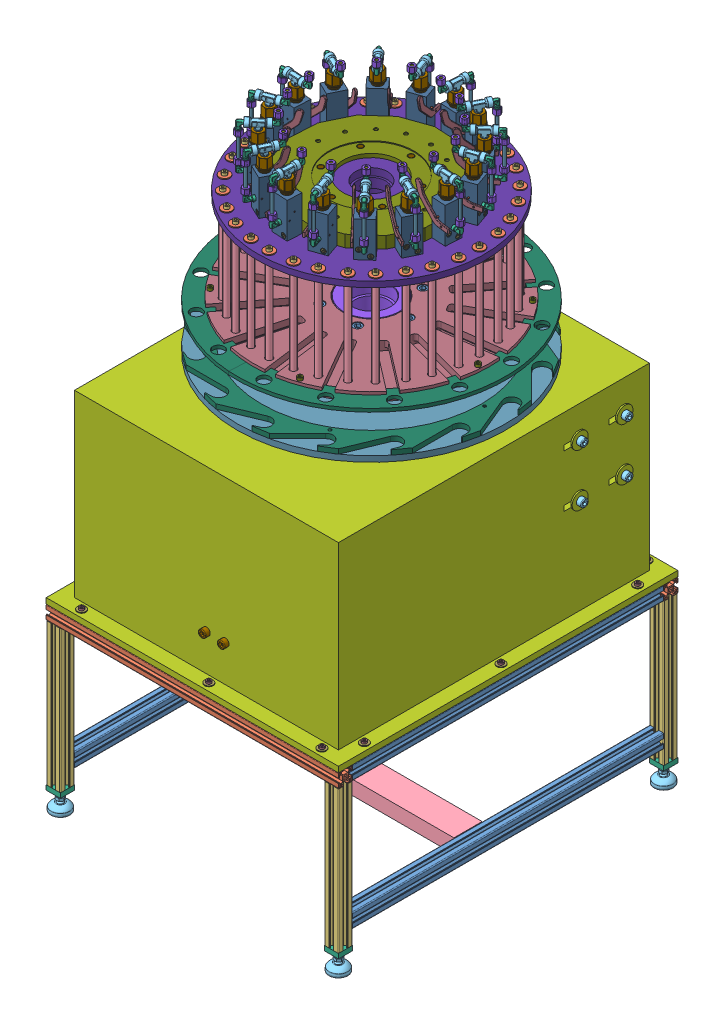
SolidWorks assembly Assieme_FINALE, configuration Default. Lengths in mm.
Overall size (778.63 1264.83 778.63).
659 component instances, 53 part files, 36 mates.
Components (placement in the parent):
- SupportoBase_Totale-2: SupportoBase_Totale [Default] at (4.0127 -14.4529 -3.9361) x (0 1 0) z (0 0 1) size (801.2 636.12 736.12)
  - Supporto_base_macchina-1: Supporto_base_macchina [Default] at origin size (378.2 636.12 736.12)
    - profilato_30x30_590-3: profilato_30x30_590 [Default] at (275.414 713.7262 -66.645) size (30 30 660)
    - profilato_30x30_590-5: profilato_30x30_590 [Default] at (275.414 123.7262 -66.645) size (30 30 660)
    - profilato_30x30_550-5: profilato_30x30_550 [Default] at (275.414 703.7262 -716.645) x (1 0 0) z (0 1 0) size (30 30 620)
    - profilato_30x30_550-6: profilato_30x30_550 [Default] at (275.414 703.7262 -26.645) x (1 0 0) z (0 1 0) size (30 30 620)
    - profilato_30x30_272-5: profilato_30x30_272 [Default] at (-16.586 123.7262 -716.645) x (0 0 1) z (-1 0 0) size (30 30 302)
    - profilato_30x30_272-6: profilato_30x30_272 [Default] at (-16.586 713.7262 -716.645) x (0 0 1) z (-1 0 0) size (30 30 302)
    - profilato_30x30_272-7: profilato_30x30_272 [Default] at (235.414 123.7262 -26.645) x (0 0 -1) z (1 0 0) size (30 30 302)
    - profilato_30x30_272-8: profilato_30x30_272 [Default] at (-16.586 713.7262 -26.645) x (0 0 1) z (-1 0 0) size (30 30 302)
    - profilo_U_60x30_490_supporto_base_macchina-1: profilo_U_60x30_490_supporto_base_macchina [Default] at (15.1 707.7262 -323.6583) x (0 0 1) z (0 -1 0) size (60 30 569)
    - profilato_30x30_590-6: profilato_30x30_590 [Default] at (3.414 123.7262 -66.645) size (30 30 660)
    - profilato_30x30_590-7: profilato_30x30_590 [Default] at (3.414 713.7262 -676.645) x (-1 0 0) z (0 0 -1) size (30 30 660)
    - 6322125-1: 6322125 [Default] at (-85.2818 713.7262 -26.645) x (0 0 -1) z (1 0 0) size (40 40 71.2)
    - 6322125-2: 6322125 [Default] at (-85.2818 713.7262 -716.645) x (0 0 -1) z (1 0 0) size (40 40 71.2)
    - 6322125-3: 6322125 [Default] at (-85.2818 123.7262 -26.645) x (0 -0.924225 -0.381849) z (1 0 0) size (40 40 71.2)
    - 6322125-4: 6322125 [Default] at (-85.2818 123.7262 -716.645) x (0 0 -1) z (1 0 0) size (40 40 71.2)
    - tappo_filettato_Supporto_base_macchina-1: tappo_filettato_Supporto_base_macchina [Default] at (-41.586 123.7262 -26.645) x (0 0 1) z (-1 0 0) size (30 30 10.37)
    - tappo_filettato_Supporto_base_macchina-2: tappo_filettato_Supporto_base_macchina [Default] at (-41.586 123.7262 -716.645) x (0 0 1) z (-1 0 0) size (30 30 10.37)
    - tappo_filettato_Supporto_base_macchina-3: tappo_filettato_Supporto_base_macchina [Default] at (-41.586 713.7262 -716.645) x (0 0 1) z (-1 0 0) size (30 30 10.37)
    - tappo_filettato_Supporto_base_macchina-4: tappo_filettato_Supporto_base_macchina [Default] at (-51.586 713.7262 -26.645) x (0 0 -1) z (1 0 0) size (30 30 10.37)
  - assieme_base-1: assieme_base [Default] at (466.8009 1138.7262 -472.0974) x (0 0 -1) z (0 -1 0) size (720 423 620)
    - Supporto di Base per macchina-1: Supporto di Base per macchina [Default] at (-460.4524 -176.3869 1030) size (720 403 620)
    - canotto di supporto-1: canotto di supporto [Default] at (-100.4524 134.8265 740) x (0 1 0) z (-0.866025 0 0.5) size (220 238 238)
    - m10 35mm-7: m10 35mm [ISO 4762 M10 x 35 - 35N] at (4.5476 246.6131 740) x (0 -1 0) z (1 0 0) size (45 16 16)
    - m10 35mm-8: m10 35mm [ISO 4762 M10 x 35 - 35N] at (-47.9524 246.6131 649.0673) x (0 -1 0) z (0.5 0 -0.866025) size (45 16 16)
    - m10 35mm-9: m10 35mm [ISO 4762 M10 x 35 - 35N] at (-152.9524 246.6131 649.0673) x (0 -1 0) z (-0.5 0 -0.866025) size (45 16 16)
    - m10 35mm-10: m10 35mm [ISO 4762 M10 x 35 - 35N] at (-205.4524 246.6131 740) x (0 -1 0) z (-1 0 0) size (45 16 16)
    - m10 35mm-11: m10 35mm [ISO 4762 M10 x 35 - 35N] at (-152.9524 246.6131 830.9327) x (0 -1 0) z (-0.5 0 0.866025) size (45 16 16)
    - m10 35mm-12: m10 35mm [ISO 4762 M10 x 35 - 35N] at (-47.9524 246.6131 830.9327) x (0 -1 0) z (0.5 0 0.866025) size (45 16 16)
    - Traversa di blocco albero-1: Traversa di blocco albero [Default] at (-100.4524 -86.3869 772.5) size (644 42 65)
    - m10 35mm-13: m10 35mm [ISO 4762 M10 x 35 - 35N] at (239.5476 -86.3869 760) x (-1 0 0) z (0 -1 0) size (45 16 16)
    - m10 35mm-16: m10 35mm [ISO 4762 M10 x 35 - 35N] at (239.5476 -86.3869 720) x (-1 0 0) z (0 -1 0) size (45 16 16)
    - m10 35mm-17: m10 35mm [ISO 4762 M10 x 35 - 35N] at (-440.4524 -86.3869 720) x (1 0 0) z (0 1 0) size (45 16 16)
    - m10 35mm-18: m10 35mm [ISO 4762 M10 x 35 - 35N] at (-440.4524 -86.3869 760) x (1 0 0) z (0 1 0) size (45 16 16)
  - DadoT-2: DadoT [Default] at (288.4104 668.7262 -716.645) x (0 0 -1) z (0 -1 0) size (16.5 6 8)
  - DadoT-9: DadoT [Default] at (288.4104 668.7262 -26.645) x (0 0 -1) z (0 -1 0) size (16.5 6 8)
  - DadoT-10: DadoT [Default] at (288.6104 713.7262 -661.645) x (0 1 0) z (0 0 -1) size (16.5 6 8)
  - DadoT-11: DadoT [Default] at (288.6104 713.7262 -371.645) x (0 1 0) z (0 0 -1) size (16.5 6 8)
  - DadoT-12: DadoT [Default] at (288.6104 713.7262 -81.645) x (0 1 0) z (0 0 -1) size (16.5 6 8)
  - DadoT-13: DadoT [Default] at (288.6104 123.7262 -661.645) x (0 1 0) z (0 0 -1) size (16.5 6 8)
  - DadoT-15: DadoT [Default] at (288.6104 123.7262 -371.645) x (0 1 0) z (0 0 -1) size (16.5 6 8)
  - DadoT-17: DadoT [Default] at (288.6104 123.7262 -81.645) x (0 1 0) z (0 0 -1) size (16.5 6 8)
  - RosettaM6-1: RosettaM6 [Washer ISO 7093 - 6] at (302.414 713.7262 -661.645) x (-1 0 0) z (0 0 1) size (1.6 18 18)
  - ViteM6-20-1: ViteM6-20 [ISO 4762 M6 x 20 - 20S] at (308.414 713.7262 -661.645) x (-1 0 0) z (0 0 1) size (26 10 10)
  - RosettaM6-2: RosettaM6 [Washer ISO 7093 - 6] at (302.414 668.7262 -716.645) x (-1 0 0) z (0 0 1) size (1.6 18 18)
  - ViteM6-20-2: ViteM6-20 [ISO 4762 M6 x 20 - 20S] at (308.414 668.7262 -716.645) x (-1 0 0) z (0 0 1) size (26 10 10)
  - RosettaM6-3: RosettaM6 [Washer ISO 7093 - 6] at (302.414 713.7262 -371.645) x (-1 0 0) z (0 0 1) size (1.6 18 18)
  - RosettaM6-4: RosettaM6 [Washer ISO 7093 - 6] at (302.414 713.7262 -81.645) x (-1 0 0) z (0 0 1) size (1.6 18 18)
  - ViteM6-20-3: ViteM6-20 [ISO 4762 M6 x 20 - 20S] at (308.414 713.7262 -371.645) x (-1 0 0) z (0 0 1) size (26 10 10)
  - ViteM6-20-4: ViteM6-20 [ISO 4762 M6 x 20 - 20S] at (308.414 713.7262 -81.645) x (-1 0 0) z (0 0 1) size (26 10 10)
  - RosettaM6-5: RosettaM6 [Washer ISO 7093 - 6] at (302.414 123.7262 -661.645) x (-1 0 0) z (0 0 1) size (1.6 18 18)
  - ViteM6-20-5: ViteM6-20 [ISO 4762 M6 x 20 - 20S] at (308.414 123.7262 -661.645) x (-1 0 0) z (0 0 1) size (26 10 10)
  - RosettaM6-6: RosettaM6 [Washer ISO 7093 - 6] at (302.414 123.7262 -371.645) x (-1 0 0) z (0 0 1) size (1.6 18 18)
  - RosettaM6-7: RosettaM6 [Washer ISO 7093 - 6] at (302.414 123.7262 -81.645) x (-1 0 0) z (0 0 1) size (1.6 18 18)
  - ViteM6-20-6: ViteM6-20 [ISO 4762 M6 x 20 - 20S] at (308.414 123.7262 -371.645) x (-1 0 0) z (0 0 1) size (26 10 10)
  - ViteM6-20-7: ViteM6-20 [ISO 4762 M6 x 20 - 20S] at (308.414 123.7262 -81.645) x (-1 0 0) z (0 0 1) size (26 10 10)
  - ViteM6-20-8: ViteM6-20 [ISO 4762 M6 x 20 - 20S] at (308.414 398.7262 -716.645) x (-1 0 0) z (0 0 1) size (26 10 10)
  - RosettaM6-8: RosettaM6 [Washer ISO 7093 - 6] at (302.414 398.7262 -716.645) x (-1 0 0) z (0 0 1) size (1.6 18 18)
  - DadoT-19: DadoT [Default] at (288.4104 398.7262 -716.645) x (0 0 -1) z (0 -1 0) size (16.5 6 8)
  - DadoT-20: DadoT [Default] at (288.4104 158.7262 -716.645) x (0 0 -1) z (0 -1 0) size (16.5 6 8)
  - RosettaM6-9: RosettaM6 [Washer ISO 7093 - 6] at (302.414 158.7262 -716.645) x (-1 0 0) z (0 0 1) size (1.6 18 18)
  - ViteM6-20-9: ViteM6-20 [ISO 4762 M6 x 20 - 20S] at (308.414 158.7262 -716.645) x (-1 0 0) z (0 0 1) size (26 10 10)
  - DadoT-21: DadoT [Default] at (288.4104 668.7262 -26.645) x (0 0 -1) z (0 -1 0) size (16.5 6 8)
  - RosettaM6-10: RosettaM6 [Washer ISO 7093 - 6] at (302.414 668.7262 -26.645) x (-1 0 0) z (0 0 1) size (1.6 18 18)
  - ViteM6-20-10: ViteM6-20 [ISO 4762 M6 x 20 - 20S] at (308.414 668.7262 -26.645) x (-1 0 0) z (0 0 1) size (26 10 10)
  - DadoT-22: DadoT [Default] at (288.4104 158.7262 -26.645) x (0 0 -1) z (0 -1 0) size (16.5 6 8)
  - RosettaM6-11: RosettaM6 [Washer ISO 7093 - 6] at (302.414 158.7262 -26.645) x (-1 0 0) z (0 0 1) size (1.6 18 18)
  - ViteM6-20-11: ViteM6-20 [ISO 4762 M6 x 20 - 20S] at (308.414 158.7262 -26.645) x (-1 0 0) z (0 0 1) size (26 10 10)
  - ViteM6-20-12: ViteM6-20 [ISO 4762 M6 x 20 - 20S] at (308.414 398.7262 -26.645) x (-1 0 0) z (0 0 1) size (26 10 10)
  - RosettaM6-12: RosettaM6 [Washer ISO 7093 - 6] at (302.414 398.7262 -26.645) x (-1 0 0) z (0 0 1) size (1.6 18 18)
  - DadoT-23: DadoT [Default] at (288.4104 398.7262 -26.645) x (0 0 -1) z (0 -1 0) size (16.5 6 8)
- motoriduttore-1: motoriduttore [Default] at (-164.7135 275.9611 -1179.5811) x (0 0 1) z (-1 0 0) size (200 160 175)
- Assieme_Riduttore-1: Assieme_Riduttore [Default] at (-346.4148 520.923 -401.8673) x (0 1 0) z (0.342115 0 -0.939658) size (226 168.82 169.04)
  - AlberoRiduttore-1: AlberoRiduttore [Default] at (-61.6906 7.4655 211) size (201 29 29)
  - linguetta_uni6604_b_8x7x50-1: linguetta_uni6604_b_8x7x50 [Default] at (-116.7419 7.4655 226) x (1 0 0) z (0 1 0) size (50 7 8)
  - linguetta_uni6604_b_8x7x35-1: linguetta_uni6604_b_8x7x35 [Default] at (-33.7419 7.4655 226.5) x (1 0 0) z (0 1 0) size (35 7 8)
  - linguetta_uni6604_b_8x7x35-2: linguetta_uni6604_b_8x7x35 [Default] at (41.2581 7.4655 226.5) x (1 0 0) z (0 1 0) size (35 7 8)
  - ASSIEME-LASS-90-VERS-B-O-25-3D.step-1: ASSIEME-LASS-90-VERS-B-O-25-3D.step [Default] at (-111.3519 -70.5563 279.3493) x (-1 0 0) z (0 0.707107 -0.707107) size (64.28 105 105)
  - Rondella di fermo-1: Rondella di fermo [Default] at (-122.7419 7.4655 211) x (0 0.707107 -0.707107) z (-1 0 0) size (36 36 3)
  - M8 25 mm-1: M8 25 mm [ISO 4762 M8 x 25 - 25N] at (92.2581 7.4655 211) x (-1 0 0) z (0 1 0) size (33 13 13)
  - M8 25 mm-2: M8 25 mm [ISO 4762 M8 x 25 - 25N] at (-133.7419 7.4655 211) x (1 0 0) z (0 -0.707107 0.707107) size (33 13 13)
  - M6 16mm-3: M6 16mm [ISO 4762 M6 x 16 - 16N] at (-44.8119 40.5589 196.8286) x (-1 0 0) z (0 0.935687 0.352831) size (22 10 10)
  - M6 16mm-14: M6 16mm [ISO 4762 M6 x 16 - 16N] at (-44.8119 11.7394 175.2546) x (-1 0 0) z (0 0.773404 -0.633913) size (22 10 10)
  - M6 16mm-15: M6 16mm [ISO 4762 M6 x 16 - 16N] at (-44.8119 -21.354 189.426) x (-1 0 0) z (0 -0.162283 -0.986744) size (22 10 10)
  - M6 16mm-16: M6 16mm [ISO 4762 M6 x 16 - 16N] at (-44.8119 -25.6279 225.1714) x (-1 0 0) z (0 -0.935687 -0.352831) size (22 10 10)
  - M6 16mm-17: M6 16mm [ISO 4762 M6 x 16 - 16N] at (-44.8119 3.1916 246.7454) x (-1 0 0) z (0 -0.773404 0.633913) size (22 10 10)
  - M6 16mm-18: M6 16mm [ISO 4762 M6 x 16 - 16N] at (-44.8119 36.285 232.574) x (-1 0 0) z (0 0.162283 0.986744) size (22 10 10)
  - Parte1^Assieme_Riduttore-1: Parte1^Assieme_Riduttore [Default] at origin (virtual)
  - ruota dentata m22-4: ruota dentata m22 [Chain wheel ISO - 22Z 10A-1 --22SA36.0N] at (-59.7419 7.4655 211) x (1 0 0) z (0 -0.599278 0.800541) size (8.93 120.13 121.23)
  - Rondella di fermo-2: Rondella di fermo [Default] at (84.2581 7.4655 211) x (0 0 1) z (-1 0 0) size (36 36 3)
- socket head cap screw_iso-1: socket head cap screw_iso [ISO 4762 M10 x 40 - 40N] at (-121.7135 603.4611 -555.5811) x (-1 0 0) z (0 -0.924225 -0.381849) size (50 16 16)
- socket head cap screw_iso-2: socket head cap screw_iso [ISO 4762 M10 x 40 - 40N] at (-121.7135 492.4611 -555.5811) x (-1 0 0) z (0 0 1) size (50 16 16)
- socket head cap screw_iso-3: socket head cap screw_iso [ISO 4762 M10 x 40 - 40N] at (-121.7135 603.4611 -650.5811) x (-1 0 0) z (0 0 1) size (50 16 16)
- socket head cap screw_iso-4: socket head cap screw_iso [ISO 4762 M10 x 40 - 40N] at (-121.7135 492.4611 -650.5811) x (-1 0 0) z (0 0 1) size (50 16 16)
- hex nut style 2 gradeab_iso-1: hex nut style 2 gradeab_iso [ISO - 4033 - M10 - W - N] at (-174.0135 603.4611 -650.5811) x (0 0 1) z (-1 0 0) size (16 18.48 9.3)
- hex nut style 2 gradeab_iso-2: hex nut style 2 gradeab_iso [ISO - 4033 - M10 - W - N] at (-174.0135 603.4611 -555.5811) x (0 0 1) z (-1 0 0) size (16 18.48 9.3)
- hex nut style 2 gradeab_iso-3: hex nut style 2 gradeab_iso [ISO - 4033 - M10 - W - N] at (-174.0135 492.4611 -650.5811) x (0 0 1) z (-1 0 0) size (16 18.48 9.3)
- hex nut style 2 gradeab_iso-4: hex nut style 2 gradeab_iso [ISO - 4033 - M10 - W - N] at (-174.0135 492.4611 -555.5811) x (0 0 1) z (-1 0 0) size (16 18.48 9.3)
- plain washer xlarge grade c_iso-1: plain washer xlarge grade c_iso [Washer ISO 7094 - 10] at (-134.7135 603.4611 -555.5811) x (-1 0 0) z (0 0.924225 0.381849) size (3 34 34)
- plain washer xlarge grade c_iso-2: plain washer xlarge grade c_iso [Washer ISO 7094 - 10] at (-134.7135 492.4611 -555.5811) x (-1 0 0) z (0 0 1) size (3 34 34)
- plain washer xlarge grade c_iso-3: plain washer xlarge grade c_iso [Washer ISO 7094 - 10] at (-134.7135 492.4611 -650.5811) x (-1 0 0) z (0 0 1) size (3 34 34)
- plain washer xlarge grade c_iso-4: plain washer xlarge grade c_iso [Washer ISO 7094 - 10] at (-134.7135 603.4611 -650.5811) x (-1 0 0) z (0 0 1) size (3 34 34)
- assieme parte rotante-1: assieme parte rotante [Default] at (-376.3498 623.9178 -790.5811) x (0 1 0) z (0 0 1) size (749.63 778.63 778.63)
  - albero rotazione piatti-1: albero rotazione piatti [Default] at (60.413 18.3637 415) size (415 200 200)
  - seger 100mm-1: seger 100mm [KS 1336 E - 100] at (-146.4567 18.3637 415) x (0 0 -1) z (1 0 0) size (107.55 112.98 3)
  - SKF - 6020 - 20,DE,NC,20_68-1: SKF - 6020 - 20,DE,NC,20_68 [SKF - 6020 - 20,DE,NC,20_68] at (-131.4567 18.3637 415) x (1 0 0) z (0 -0.434476 -0.900684) size (24 150 150)
  - calettatore d95-1: calettatore d95 [Default] at (-173.8867 18.3637 415) size (39.5 135 135)
  - Chain wheel ISO - 50Z 10A-1-1: Chain wheel ISO - 50Z 10A-1 [Chain wheel ISO - 50Z 10A-1 --50SB120H25L95.0N] at (-164.8867 18.3637 415) size (28.93 262.06 262.51)
  - Disco supporto montaggio e Colonne-1: Disco supporto montaggio e Colonne [Default] at (204.0433 18.3637 415) x (0 -0.866025 -0.5) z (1 0 0) size (499.6 499.6 29)
  - SKF - 6020 - 20,DE,NC,20_68-2: SKF - 6020 - 20,DE,NC,20_68 [SKF - 6020 - 20,DE,NC,20_68] at (62.0433 18.3637 415) x (1 0 0) z (0 -0.432628 -0.901573) size (24 150 150)
  - piatto rotante porta tappi-1: piatto rotante porta tappi [Default] at (99.0433 18.3637 415) x (0 0 -1) z (1 0 0) size (570 570 20.57)
  - disco trasportatore tappi 31-1: disco trasportatore tappi 31 [Default] at (111.0433 18.3637 415) x (0 0.5 -0.866025) z (1 0 0) size (570 570 10.42)
  - Distributore Rotante-1: Distributore Rotante [Default] at (425.0433 18.3637 415) x (0 -0.055301 -0.99847) z (1 0 0) size (310 310 25.54)
  - disco trascinato porta distributore vuoto-1: disco trascinato porta distributore vuoto [Default] at (400.0433 18.3637 415) x (0 0.055301 0.99847) z (-1 0 0) size (480 480 50)
  - m12 35mm-1: m12 35mm [ISO 4762 M12 x 35 - 35N] at (376.0433 -53.0243 378.8925) x (1 0 0) z (0 -0.5 0.866025) size (47 18 18)
  - m12 90mm-3: m12 90mm [ISO 4762 M12 x 90 - 90N] at (203.0433 -21.6363 345.718) x (-1 0 0) z (0 -0.5 0.866025) size (102 18 18)
  - rondella m6 22mm-1: rondella m6 22mm [Washer ISO 7094 - 6] at (99.0433 -101.6363 207.1539) x (1 0 0) z (0 -1 0) size (2 22 22)
  - M6 20mm-1: M6 20mm [ISO 4762 M6 x 20 - 20N] at (91.0433 -101.6363 207.1539) x (1 0 0) z (0 0.5 0.866025) size (26 10 10)
  - m12 35mm-2: m12 35mm [ISO 4762 M12 x 35 - 35N] at (376.0433 13.9397 335.1224) x (1 0 0) z (0 -1 0) size (47 18 18)
  - m12 35mm-3: m12 35mm [ISO 4762 M12 x 35 - 35N] at (376.0433 85.3277 371.2299) x (1 0 0) z (0 -0.5 -0.866025) size (47 18 18)
  - m12 35mm-4: m12 35mm [ISO 4762 M12 x 35 - 35N] at (376.0433 89.7517 451.1075) x (1 0 0) z (0 0.5 -0.866025) size (47 18 18)
  - m12 35mm-5: m12 35mm [ISO 4762 M12 x 35 - 35N] at (376.0433 22.7877 494.8776) x (1 0 0) z (0 1 0) size (47 18 18)
  - m12 35mm-6: m12 35mm [ISO 4762 M12 x 35 - 35N] at (376.0433 -48.6003 458.7701) x (1 0 0) z (0 0.5 0.866025) size (47 18 18)
  - rondella m6 22mm-2: rondella m6 22mm [Washer ISO 7094 - 6] at (99.0433 138.3637 207.1539) x (1 0 0) z (0 -0.5 -0.866025) size (2 22 22)
  - rondella m6 22mm-3: rondella m6 22mm [Washer ISO 7094 - 6] at (99.0433 258.3637 415) x (1 0 0) z (0 0.5 -0.866025) size (2 22 22)
  - rondella m6 22mm-4: rondella m6 22mm [Washer ISO 7094 - 6] at (99.0433 138.3637 622.8461) x (1 0 0) z (0 1 0) size (2 22 22)
  - rondella m6 22mm-5: rondella m6 22mm [Washer ISO 7094 - 6] at (99.0433 -101.6363 622.8461) x (1 0 0) z (0 0.5 0.866025) size (2 22 22)
  - rondella m6 22mm-6: rondella m6 22mm [Washer ISO 7094 - 6] at (99.0433 -221.6363 415) x (1 0 0) z (0 -0.5 0.866025) size (2 22 22)
  - M6 20mm-2: M6 20mm [ISO 4762 M6 x 20 - 20N] at (91.0433 138.3637 207.1539) x (1 0 0) z (0 -0.5 0.866025) size (26 10 10)
  - M6 20mm-3: M6 20mm [ISO 4762 M6 x 20 - 20N] at (91.0433 258.3637 415) x (1 0 0) z (0 -1 0) size (26 10 10)
  - M6 20mm-4: M6 20mm [ISO 4762 M6 x 20 - 20N] at (91.0433 138.3637 622.8461) x (1 0 0) z (0 -0.5 -0.866025) size (26 10 10)
  - M6 20mm-5: M6 20mm [ISO 4762 M6 x 20 - 20N] at (91.0433 -101.6363 622.8461) x (1 0 0) z (0 0.5 -0.866025) size (26 10 10)
  - M6 20mm-6: M6 20mm [ISO 4762 M6 x 20 - 20N] at (91.0433 -221.6363 415) x (1 0 0) z (0 1 0) size (26 10 10)
  - m12 90mm-4: m12 90mm [ISO 4762 M12 x 90 - 90N] at (203.0433 58.3637 345.718) x (-1 0 0) z (0 -1 0) size (102 18 18)
  - m12 90mm-5: m12 90mm [ISO 4762 M12 x 90 - 90N] at (203.0433 98.3637 415) x (-1 0 0) z (0 -0.5 -0.866025) size (102 18 18)
  - m12 90mm-6: m12 90mm [ISO 4762 M12 x 90 - 90N] at (203.0433 58.3637 484.282) x (-1 0 0) z (0 0.5 -0.866025) size (102 18 18)
  - m12 90mm-7: m12 90mm [ISO 4762 M12 x 90 - 90N] at (203.0433 -21.6363 484.282) x (-1 0 0) z (0 1 0) size (102 18 18)
  - m12 90mm-8: m12 90mm [ISO 4762 M12 x 90 - 90N] at (203.0433 -61.6363 415) x (-1 0 0) z (0 0.5 0.866025) size (102 18 18)
  - asta scorrimento carello-1: asta scorrimento carello [Default] at (287.5433 70.1437 197.9013) x (0 0 -1) z (1 0 0) size (12 12 225)
  - rondella m6 22mm-7: rondella m6 22mm [Washer ISO 7094 - 6] at (175.0433 70.1437 197.9013) x (1 0 0) z (0 -1 0) size (2 22 22)
  - M6 16mm-1: M6 16mm [ISO 4762 M6 x 16 - 16N] at (167.0433 70.1437 197.9013) size (22 10 10)
  - M6 16mm-2: M6 16mm [ISO 4762 M6 x 16 - 16N] at (408.0433 70.1437 197.9013) x (-1 0 0) z (0 0 -1) size (22 10 10)
  - rondella m6 22mm-8: rondella m6 22mm [Washer ISO 7094 - 6] at (400.0433 70.1437 197.9013) x (-1 0 0) z (0 1 0) size (2 22 22)
  - rondella m6 22mm-9: rondella m6 22mm [Washer ISO 7094 - 6] at (175.0433 24.5373 191.8971) x (1 0 0) z (0 -0.965926 -0.258819) size (2 22 22)
  - M6 16mm-3: M6 16mm [ISO 4762 M6 x 16 - 16N] at (167.0433 24.5373 191.8971) x (1 0 0) z (0 0.258819 -0.965926) size (22 10 10)
  - asta scorrimento carello-2: asta scorrimento carello [Default] at (287.5433 24.5373 191.8971) x (0 0.258819 -0.965926) z (-1 0 0) size (12 12 225)
  - rondella m6 22mm-10: rondella m6 22mm [Washer ISO 7094 - 6] at (400.0433 24.5373 191.8971) x (-1 0 0) z (0 0.965926 0.258819) size (2 22 22)
  - M6 16mm-4: M6 16mm [ISO 4762 M6 x 16 - 16N] at (408.0433 24.5373 191.8971) x (-1 0 0) z (0 -0.258819 0.965926) size (22 10 10)
  - AssiemeValvola-1: AssiemeValvola [Default] at (515.3257 74.6348 254.5832) x (0 -0.331007 0.943628) z (0 0.943628 0.331007) size (90.26 138.63 38)
    - RaccordoT-1: RaccordoT [Default] at origin size (43 29.75 16.5)
    - Raccordo a L-1: Raccordo a L [Default] at (-30 0 0) x (0 -1 0) z (0 0 -1) size (28.34 25.51 14.01)
      - 1809_06_10_01-1: 1809_06_10_01 [Default] at origin size (22.49 23 10)
      - 1809_06_10_02-1: 1809_06_10_02 [Default] at origin size (6.5 8.5 8.5)
      - 1809_06_10_03-1: 1809_06_10_03 [Default] at origin size (11.02 15.01 14.01)
    - Raccordo a L-2: Raccordo a L [Default] at (30 0 0) x (0 1 0) z (0 0 -1) size (28.34 25.51 14.01)
      - 1809_06_10_01-1: 1809_06_10_01 [Default] at origin size (22.49 23 10)
      - 1809_06_10_02-1: 1809_06_10_02 [Default] at origin size (6.5 8.5 8.5)
      - 1809_06_10_03-1: 1809_06_10_03 [Default] at origin size (11.02 15.01 14.01)
    - TappoChiusura-1: TappoChiusura [Default] at (0 -32 0) x (0 -1 0) z (0 0 1) size (38.28 26.74 26.74)
    - CorpoValvola-1: CorpoValvola [Default] at (-15 -115.2824 0) size (30 75 34)
    - Raccordo a L-3: Raccordo a L [Default] at (-30 -88.2824 0) x (0 1 0) z (0 0 1) size (28.34 25.51 14.01)
      - 1809_06_10_01-1: 1809_06_10_01 [Default] at origin size (22.49 23 10)
      - 1809_06_10_02-1: 1809_06_10_02 [Default] at origin size (6.5 8.5 8.5)
      - 1809_06_10_03-1: 1809_06_10_03 [Default] at origin size (11.02 15.01 14.01)
    - Spina_3x38-1: Spina_3x38 [Default] at (0 -68.2824 -21) x (-1 0 0) z (0 0 1) size (3 3 38)
    - Spina_3x38-2: Spina_3x38 [Default] at (-10 -80.2824 -21) x (0.996193 0.087174 0) z (0 0 1) size (3 3 38)
    - M5 40mm-3: M5 40mm [ISO 4762 M5 x 40 - 40N] at (-14.6 -108.7824 9) size (45 8.5 8.5)
    - M5 40mm-2: M5 40mm [ISO 4762 M5 x 40 - 40N] at (-14.6 -96.7824 -9) size (45 8.5 8.5)
    - LevaValvola-1: LevaValvola [Default] at (-24.507 -86.571 -17) x (0.996193 0.087174 0) z (0 0 1) size (77.55 60.2 4)
    - Tubo-1: Tubo [Default] at (-30 -15.9665 0) x (1 0 0) z (0 -1 0) size (6 6 56.4)
  - M6 16mm-5: M6 16mm [ISO 4762 M6 x 16 - 16N] at (167.0433 -16.8778 194.6116) x (1 0 0) z (0 0.382683 0.92388) size (22 10 10)
  - M6 16mm-6: M6 16mm [ISO 4762 M6 x 16 - 16N] at (167.0433 -98.5342 224.874) x (1 0 0) z (0 0.707107 0.707107) size (22 10 10)
  - M6 16mm-7: M6 16mm [ISO 4762 M6 x 16 - 16N] at (167.0433 -162.3939 284.0814) x (1 0 0) z (0 0.92388 0.382683) size (22 10 10)
  - M6 16mm-8: M6 16mm [ISO 4762 M6 x 16 - 16N] at (167.0433 -198.735 363.22) x (1 0 0) z (0 1 0) size (22 10 10)
  - M6 16mm-9: M6 16mm [ISO 4762 M6 x 16 - 16N] at (167.0433 -202.0247 450.2415) x (1 0 0) z (0 0.92388 -0.382683) size (22 10 10)
  - M6 16mm-10: M6 16mm [ISO 4762 M6 x 16 - 16N] at (167.0433 -171.7623 531.8979) x (1 0 0) z (0 0.707107 -0.707107) size (22 10 10)
  - M6 16mm-11: M6 16mm [ISO 4762 M6 x 16 - 16N] at (167.0433 -112.5549 595.7576) x (1 0 0) z (0 0.382683 -0.92388) size (22 10 10)
  - M6 16mm-12: M6 16mm [ISO 4762 M6 x 16 - 16N] at (167.0433 -33.4163 632.0987) x (1 0 0) z (0 0 -1) size (22 10 10)
  - M6 16mm-13: M6 16mm [ISO 4762 M6 x 16 - 16N] at (167.0433 53.6052 635.3884) x (1 0 0) z (0 -0.382683 -0.92388) size (22 10 10)
  - M6 16mm-14: M6 16mm [ISO 4762 M6 x 16 - 16N] at (167.0433 135.2616 605.126) x (1 0 0) z (0 -0.707107 -0.707107) size (22 10 10)
  - M6 16mm-15: M6 16mm [ISO 4762 M6 x 16 - 16N] at (167.0433 199.1213 545.9186) x (1 0 0) z (0 -0.92388 -0.382683) size (22 10 10)
  - M6 16mm-16: M6 16mm [ISO 4762 M6 x 16 - 16N] at (167.0433 235.4624 466.78) x (1 0 0) z (0 -1 0) size (22 10 10)
  - M6 16mm-17: M6 16mm [ISO 4762 M6 x 16 - 16N] at (167.0433 238.7521 379.7585) x (1 0 0) z (0 -0.92388 0.382683) size (22 10 10)
  - M6 16mm-18: M6 16mm [ISO 4762 M6 x 16 - 16N] at (167.0433 208.4897 298.1021) x (1 0 0) z (0 -0.707107 0.707107) size (22 10 10)
  - M6 16mm-19: M6 16mm [ISO 4762 M6 x 16 - 16N] at (167.0433 149.2823 234.2424) x (1 0 0) z (0 -0.382683 0.92388) size (22 10 10)
  - rondella m6 22mm-11: rondella m6 22mm [Washer ISO 7094 - 6] at (175.0433 -16.8778 194.6116) x (1 0 0) z (0 -0.92388 0.382683) size (2 22 22)
  - rondella m6 22mm-12: rondella m6 22mm [Washer ISO 7094 - 6] at (175.0433 -98.5342 224.874) x (1 0 0) z (0 -0.707107 0.707107) size (2 22 22)
  - rondella m6 22mm-13: rondella m6 22mm [Washer ISO 7094 - 6] at (175.0433 -162.3939 284.0814) x (1 0 0) z (0 -0.382683 0.92388) size (2 22 22)
  - rondella m6 22mm-14: rondella m6 22mm [Washer ISO 7094 - 6] at (175.0433 -198.735 363.22) size (2 22 22)
  - rondella m6 22mm-15: rondella m6 22mm [Washer ISO 7094 - 6] at (175.0433 -202.0247 450.2415) x (1 0 0) z (0 0.382683 0.92388) size (2 22 22)
  - rondella m6 22mm-16: rondella m6 22mm [Washer ISO 7094 - 6] at (175.0433 -171.7623 531.8979) x (1 0 0) z (0 0.707107 0.707107) size (2 22 22)
  - rondella m6 22mm-17: rondella m6 22mm [Washer ISO 7094 - 6] at (175.0433 -112.5549 595.7576) x (1 0 0) z (0 0.92388 0.382683) size (2 22 22)
  - rondella m6 22mm-18: rondella m6 22mm [Washer ISO 7094 - 6] at (175.0433 -33.4163 632.0987) x (1 0 0) z (0 1 0) size (2 22 22)
  - rondella m6 22mm-19: rondella m6 22mm [Washer ISO 7094 - 6] at (175.0433 53.6052 635.3884) x (1 0 0) z (0 0.92388 -0.382683) size (2 22 22)
  - rondella m6 22mm-20: rondella m6 22mm [Washer ISO 7094 - 6] at (175.0433 135.2616 605.126) x (1 0 0) z (0 0.707107 -0.707107) size (2 22 22)
  - rondella m6 22mm-21: rondella m6 22mm [Washer ISO 7094 - 6] at (175.0433 199.1213 545.9186) x (1 0 0) z (0 0.382683 -0.92388) size (2 22 22)
  - rondella m6 22mm-22: rondella m6 22mm [Washer ISO 7094 - 6] at (175.0433 235.4624 466.78) x (1 0 0) z (0 0 -1) size (2 22 22)
  - rondella m6 22mm-23: rondella m6 22mm [Washer ISO 7094 - 6] at (175.0433 238.7521 379.7585) x (1 0 0) z (0 -0.382683 -0.92388) size (2 22 22)
  - rondella m6 22mm-24: rondella m6 22mm [Washer ISO 7094 - 6] at (175.0433 208.4897 298.1021) x (1 0 0) z (0 -0.707107 -0.707107) size (2 22 22)
  - rondella m6 22mm-25: rondella m6 22mm [Washer ISO 7094 - 6] at (175.0433 149.2823 234.2424) x (1 0 0) z (0 -0.92388 -0.382683) size (2 22 22)
  - asta scorrimento carello-3: asta scorrimento carello [Default] at (287.5433 -16.8778 194.6116) x (0 -0.382683 -0.92388) z (1 0 0) size (12 12 225)
  - asta scorrimento carello-4: asta scorrimento carello [Default] at (287.5433 -98.5342 224.874) x (0 -0.707107 -0.707107) z (1 0 0) size (12 12 225)
  - asta scorrimento carello-5: asta scorrimento carello [Default] at (287.5433 -162.3939 284.0814) x (0 -0.92388 -0.382683) z (1 0 0) size (12 12 225)
  - asta scorrimento carello-6: asta scorrimento carello [Default] at (287.5433 -198.735 363.22) x (0 -1 0) z (1 0 0) size (12 12 225)
  - asta scorrimento carello-7: asta scorrimento carello [Default] at (287.5433 -202.0247 450.2415) x (0 -0.92388 0.382683) z (1 0 0) size (12 12 225)
  - asta scorrimento carello-8: asta scorrimento carello [Default] at (287.5433 -171.7623 531.8979) x (0 -0.707107 0.707107) z (1 0 0) size (12 12 225)
  - asta scorrimento carello-9: asta scorrimento carello [Default] at (287.5433 -112.5549 595.7576) x (0 -0.382683 0.92388) z (1 0 0) size (12 12 225)
  - asta scorrimento carello-10: asta scorrimento carello [Default] at (287.5433 -33.4163 632.0987) x (0 0 1) z (1 0 0) size (12 12 225)
  - asta scorrimento carello-11: asta scorrimento carello [Default] at (287.5433 53.6052 635.3884) x (0 0.382683 0.92388) z (1 0 0) size (12 12 225)
  - asta scorrimento carello-12: asta scorrimento carello [Default] at (287.5433 135.2616 605.126) x (0 0.707107 0.707107) z (1 0 0) size (12 12 225)
  - asta scorrimento carello-13: asta scorrimento carello [Default] at (287.5433 199.1213 545.9186) x (0 0.92388 0.382683) z (1 0 0) size (12 12 225)
  - asta scorrimento carello-14: asta scorrimento carello [Default] at (287.5433 235.4624 466.78) x (0 1 0) z (1 0 0) size (12 12 225)
  - asta scorrimento carello-15: asta scorrimento carello [Default] at (287.5433 238.7521 379.7585) x (0 0.92388 -0.382683) z (1 0 0) size (12 12 225)
  - asta scorrimento carello-16: asta scorrimento carello [Default] at (287.5433 208.4897 298.1021) x (0 0.707107 -0.707107) z (1 0 0) size (12 12 225)
  - asta scorrimento carello-17: asta scorrimento carello [Default] at (287.5433 149.2823 234.2424) x (0 0.382683 -0.92388) z (1 0 0) size (12 12 225)
  - M6 16mm-20: M6 16mm [ISO 4762 M6 x 16 - 16N] at (408.0433 -16.8778 194.6116) x (-1 0 0) z (0 -0.382683 -0.92388) size (22 10 10)
  - M6 16mm-21: M6 16mm [ISO 4762 M6 x 16 - 16N] at (408.0433 -98.5342 224.874) x (-1 0 0) z (0 -0.707107 -0.707107) size (22 10 10)
  - M6 16mm-22: M6 16mm [ISO 4762 M6 x 16 - 16N] at (408.0433 -162.3939 284.0814) x (-1 0 0) z (0 -0.92388 -0.382683) size (22 10 10)
  - M6 16mm-23: M6 16mm [ISO 4762 M6 x 16 - 16N] at (408.0433 -198.735 363.22) x (-1 0 0) z (0 -1 0) size (22 10 10)
  - M6 16mm-24: M6 16mm [ISO 4762 M6 x 16 - 16N] at (408.0433 -202.0247 450.2415) x (-1 0 0) z (0 -0.92388 0.382683) size (22 10 10)
  - M6 16mm-25: M6 16mm [ISO 4762 M6 x 16 - 16N] at (408.0433 -171.7623 531.8979) x (-1 0 0) z (0 -0.707107 0.707107) size (22 10 10)
  - M6 16mm-26: M6 16mm [ISO 4762 M6 x 16 - 16N] at (408.0433 -112.5549 595.7576) x (-1 0 0) z (0 -0.382683 0.92388) size (22 10 10)
  - M6 16mm-27: M6 16mm [ISO 4762 M6 x 16 - 16N] at (408.0433 -33.4163 632.0987) x (-1 0 0) z (0 0 1) size (22 10 10)
  - M6 16mm-28: M6 16mm [ISO 4762 M6 x 16 - 16N] at (408.0433 53.6052 635.3884) x (-1 0 0) z (0 0.382683 0.92388) size (22 10 10)
  - M6 16mm-29: M6 16mm [ISO 4762 M6 x 16 - 16N] at (408.0433 135.2616 605.126) x (-1 0 0) z (0 0.707107 0.707107) size (22 10 10)
  - M6 16mm-30: M6 16mm [ISO 4762 M6 x 16 - 16N] at (408.0433 199.1213 545.9186) x (-1 0 0) z (0 0.92388 0.382683) size (22 10 10)
  - M6 16mm-31: M6 16mm [ISO 4762 M6 x 16 - 16N] at (408.0433 235.4624 466.78) x (-1 0 0) z (0 1 0) size (22 10 10)
  - M6 16mm-32: M6 16mm [ISO 4762 M6 x 16 - 16N] at (408.0433 238.7521 379.7585) x (-1 0 0) z (0 0.92388 -0.382683) size (22 10 10)
  - M6 16mm-33: M6 16mm [ISO 4762 M6 x 16 - 16N] at (408.0433 208.4897 298.1021) x (-1 0 0) z (0 0.707107 -0.707107) size (22 10 10)
  - M6 16mm-34: M6 16mm [ISO 4762 M6 x 16 - 16N] at (408.0433 149.2823 234.2424) x (-1 0 0) z (0 0.382683 -0.92388) size (22 10 10)
  - rondella m6 22mm-26: rondella m6 22mm [Washer ISO 7094 - 6] at (400.0433 -16.8778 194.6116) x (-1 0 0) z (0 0.92388 -0.382683) size (2 22 22)
  - rondella m6 22mm-27: rondella m6 22mm [Washer ISO 7094 - 6] at (400.0433 -98.5342 224.874) x (-1 0 0) z (0 0.707107 -0.707107) size (2 22 22)
  - rondella m6 22mm-28: rondella m6 22mm [Washer ISO 7094 - 6] at (400.0433 -162.3939 284.0814) x (-1 0 0) z (0 0.382683 -0.92388) size (2 22 22)
  - rondella m6 22mm-29: rondella m6 22mm [Washer ISO 7094 - 6] at (400.0433 -198.735 363.22) x (-1 0 0) z (0 0 -1) size (2 22 22)
  - rondella m6 22mm-30: rondella m6 22mm [Washer ISO 7094 - 6] at (400.0433 -202.0247 450.2415) x (-1 0 0) z (0 -0.382683 -0.92388) size (2 22 22)
  - rondella m6 22mm-31: rondella m6 22mm [Washer ISO 7094 - 6] at (400.0433 -171.7623 531.8979) x (-1 0 0) z (0 -0.707107 -0.707107) size (2 22 22)
  - rondella m6 22mm-32: rondella m6 22mm [Washer ISO 7094 - 6] at (400.0433 -112.5549 595.7576) x (-1 0 0) z (0 -0.92388 -0.382683) size (2 22 22)
  - rondella m6 22mm-33: rondella m6 22mm [Washer ISO 7094 - 6] at (400.0433 -33.4163 632.0987) x (-1 0 0) z (0 -1 0) size (2 22 22)
  - rondella m6 22mm-34: rondella m6 22mm [Washer ISO 7094 - 6] at (400.0433 53.6052 635.3884) x (-1 0 0) z (0 -0.92388 0.382683) size (2 22 22)
  - rondella m6 22mm-35: rondella m6 22mm [Washer ISO 7094 - 6] at (400.0433 135.2616 605.126) x (-1 0 0) z (0 -0.707107 0.707107) size (2 22 22)
  - rondella m6 22mm-36: rondella m6 22mm [Washer ISO 7094 - 6] at (400.0433 199.1213 545.9186) x (-1 0 0) z (0 -0.382683 0.92388) size (2 22 22)
  - rondella m6 22mm-37: rondella m6 22mm [Washer ISO 7094 - 6] at (400.0433 235.4624 466.78) x (-1 0 0) z (0 0 1) size (2 22 22)
  - rondella m6 22mm-38: rondella m6 22mm [Washer ISO 7094 - 6] at (400.0433 238.7521 379.7585) x (-1 0 0) z (0 0.382683 0.92388) size (2 22 22)
  - rondella m6 22mm-39: rondella m6 22mm [Washer ISO 7094 - 6] at (400.0433 208.4897 298.1021) x (-1 0 0) z (0 0.707107 0.707107) size (2 22 22)
  - rondella m6 22mm-40: rondella m6 22mm [Washer ISO 7094 - 6] at (400.0433 149.2823 234.2424) x (-1 0 0) z (0 0.92388 0.382683) size (2 22 22)
  - rondella m6 22mm-41: rondella m6 22mm [Washer ISO 7094 - 6] at (175.0433 -61.3104 206.5173) x (1 0 0) z (0 -0.991445 0.130526) size (2 22 22)
  - rondella m6 22mm-42: rondella m6 22mm [Washer ISO 7094 - 6] at (175.0433 -135.0285 252.8771) x (1 0 0) z (0 -0.866025 0.5) size (2 22 22)
  - rondella m6 22mm-43: rondella m6 22mm [Washer ISO 7094 - 6] at (175.0433 -185.3939 323.9186) x (1 0 0) z (0 -0.608761 0.793353) size (2 22 22)
  - rondella m6 22mm-44: rondella m6 22mm [Washer ISO 7094 - 6] at (175.0433 -204.7392 408.8264) x (1 0 0) z (0 -0.258819 0.965926) size (2 22 22)
  - rondella m6 22mm-45: rondella m6 22mm [Washer ISO 7094 - 6] at (175.0433 -190.119 494.6741) x (1 0 0) z (0 0.130526 0.991445) size (2 22 22)
  - rondella m6 22mm-46: rondella m6 22mm [Washer ISO 7094 - 6] at (175.0433 -143.7592 568.3922) x (1 0 0) z (0 0.5 0.866025) size (2 22 22)
  - rondella m6 22mm-47: rondella m6 22mm [Washer ISO 7094 - 6] at (175.0433 -72.7177 618.7576) x (1 0 0) z (0 0.793353 0.608761) size (2 22 22)
  - rondella m6 22mm-48: rondella m6 22mm [Washer ISO 7094 - 6] at (175.0433 12.1901 638.1029) x (1 0 0) z (0 0.965926 0.258819) size (2 22 22)
  - rondella m6 22mm-49: rondella m6 22mm [Washer ISO 7094 - 6] at (175.0433 98.0378 623.4827) x (1 0 0) z (0 0.991445 -0.130526) size (2 22 22)
  - rondella m6 22mm-50: rondella m6 22mm [Washer ISO 7094 - 6] at (175.0433 171.7559 577.1229) x (1 0 0) z (0 0.866025 -0.5) size (2 22 22)
  - rondella m6 22mm-51: rondella m6 22mm [Washer ISO 7094 - 6] at (175.0433 222.1213 506.0814) x (1 0 0) z (0 0.608761 -0.793353) size (2 22 22)
  - rondella m6 22mm-52: rondella m6 22mm [Washer ISO 7094 - 6] at (175.0433 241.4666 421.1736) x (1 0 0) z (0 0.258819 -0.965926) size (2 22 22)
  - rondella m6 22mm-53: rondella m6 22mm [Washer ISO 7094 - 6] at (175.0433 226.8464 335.3259) x (1 0 0) z (0 -0.130526 -0.991445) size (2 22 22)
  - rondella m6 22mm-54: rondella m6 22mm [Washer ISO 7094 - 6] at (175.0433 180.4866 261.6078) x (1 0 0) z (0 -0.5 -0.866025) size (2 22 22)
  - rondella m6 22mm-55: rondella m6 22mm [Washer ISO 7094 - 6] at (175.0433 109.4451 211.2424) x (1 0 0) z (0 -0.793353 -0.608761) size (2 22 22)
  - M6 16mm-35: M6 16mm [ISO 4762 M6 x 16 - 16N] at (167.0433 -61.3104 206.5173) x (1 0 0) z (0 -0.130526 -0.991445) size (22 10 10)
  - M6 16mm-36: M6 16mm [ISO 4762 M6 x 16 - 16N] at (167.0433 -135.0285 252.8771) x (1 0 0) z (0 -0.5 -0.866025) size (22 10 10)
  - M6 16mm-37: M6 16mm [ISO 4762 M6 x 16 - 16N] at (167.0433 -185.3939 323.9186) x (1 0 0) z (0 -0.793353 -0.608761) size (22 10 10)
  - M6 16mm-38: M6 16mm [ISO 4762 M6 x 16 - 16N] at (167.0433 -204.7392 408.8264) x (1 0 0) z (0 -0.965926 -0.258819) size (22 10 10)
  - M6 16mm-39: M6 16mm [ISO 4762 M6 x 16 - 16N] at (167.0433 -190.119 494.6741) x (1 0 0) z (0 -0.991445 0.130526) size (22 10 10)
  - M6 16mm-40: M6 16mm [ISO 4762 M6 x 16 - 16N] at (167.0433 -143.7592 568.3922) x (1 0 0) z (0 -0.866025 0.5) size (22 10 10)
  - M6 16mm-41: M6 16mm [ISO 4762 M6 x 16 - 16N] at (167.0433 -72.7177 618.7576) x (1 0 0) z (0 -0.608761 0.793353) size (22 10 10)
  - M6 16mm-42: M6 16mm [ISO 4762 M6 x 16 - 16N] at (167.0433 12.1901 638.1029) x (1 0 0) z (0 -0.258819 0.965926) size (22 10 10)
  - M6 16mm-43: M6 16mm [ISO 4762 M6 x 16 - 16N] at (167.0433 98.0378 623.4827) x (1 0 0) z (0 0.130526 0.991445) size (22 10 10)
  - M6 16mm-44: M6 16mm [ISO 4762 M6 x 16 - 16N] at (167.0433 171.7559 577.1229) x (1 0 0) z (0 0.5 0.866025) size (22 10 10)
  - M6 16mm-45: M6 16mm [ISO 4762 M6 x 16 - 16N] at (167.0433 222.1213 506.0814) x (1 0 0) z (0 0.793353 0.608761) size (22 10 10)
  - M6 16mm-46: M6 16mm [ISO 4762 M6 x 16 - 16N] at (167.0433 241.4666 421.1736) x (1 0 0) z (0 0.965926 0.258819) size (22 10 10)
  - M6 16mm-47: M6 16mm [ISO 4762 M6 x 16 - 16N] at (167.0433 226.8464 335.3259) x (1 0 0) z (0 0.991445 -0.130526) size (22 10 10)
  - M6 16mm-48: M6 16mm [ISO 4762 M6 x 16 - 16N] at (167.0433 180.4866 261.6078) x (1 0 0) z (0 0.866025 -0.5) size (22 10 10)
  - M6 16mm-49: M6 16mm [ISO 4762 M6 x 16 - 16N] at (167.0433 109.4451 211.2424) x (1 0 0) z (0 0.608761 -0.793353) size (22 10 10)
  - asta scorrimento carello-18: asta scorrimento carello [Default] at (287.5433 -61.3104 206.5173) x (0 -0.130526 -0.991445) z (-1 0 0) size (12 12 225)
  - asta scorrimento carello-19: asta scorrimento carello [Default] at (287.5433 -135.0285 252.8771) x (0 -0.5 -0.866025) z (-1 0 0) size (12 12 225)
  - asta scorrimento carello-20: asta scorrimento carello [Default] at (287.5433 -185.3939 323.9186) x (0 -0.793353 -0.608761) z (-1 0 0) size (12 12 225)
  - asta scorrimento carello-21: asta scorrimento carello [Default] at (287.5433 -204.7392 408.8264) x (0 -0.965926 -0.258819) z (-1 0 0) size (12 12 225)
  - asta scorrimento carello-22: asta scorrimento carello [Default] at (287.5433 -190.119 494.6741) x (0 -0.991445 0.130526) z (-1 0 0) size (12 12 225)
  - asta scorrimento carello-23: asta scorrimento carello [Default] at (287.5433 -143.7592 568.3922) x (0 -0.866025 0.5) z (-1 0 0) size (12 12 225)
  - asta scorrimento carello-24: asta scorrimento carello [Default] at (287.5433 -72.7177 618.7576) x (0 -0.608761 0.793353) z (-1 0 0) size (12 12 225)
  - asta scorrimento carello-25: asta scorrimento carello [Default] at (287.5433 12.1901 638.1029) x (0 -0.258819 0.965926) z (-1 0 0) size (12 12 225)
  - asta scorrimento carello-26: asta scorrimento carello [Default] at (287.5433 98.0378 623.4827) x (0 0.130526 0.991445) z (-1 0 0) size (12 12 225)
  - asta scorrimento carello-27: asta scorrimento carello [Default] at (287.5433 171.7559 577.1229) x (0 0.5 0.866025) z (-1 0 0) size (12 12 225)
  - asta scorrimento carello-28: asta scorrimento carello [Default] at (287.5433 222.1213 506.0814) x (0 0.793353 0.608761) z (-1 0 0) size (12 12 225)
  - asta scorrimento carello-29: asta scorrimento carello [Default] at (287.5433 241.4666 421.1736) x (0 0.965926 0.258819) z (-1 0 0) size (12 12 225)
  - asta scorrimento carello-30: asta scorrimento carello [Default] at (287.5433 226.8464 335.3259) x (0 0.991445 -0.130526) z (-1 0 0) size (12 12 225)
  - asta scorrimento carello-31: asta scorrimento carello [Default] at (287.5433 180.4866 261.6078) x (0 0.866025 -0.5) z (-1 0 0) size (12 12 225)
  - asta scorrimento carello-32: asta scorrimento carello [Default] at (287.5433 109.4451 211.2424) x (0 0.608761 -0.793353) z (-1 0 0) size (12 12 225)
  - rondella m6 22mm-56: rondella m6 22mm [Washer ISO 7094 - 6] at (400.0433 -61.3104 206.5173) x (-1 0 0) z (0 0.991445 -0.130526) size (2 22 22)
  - rondella m6 22mm-57: rondella m6 22mm [Washer ISO 7094 - 6] at (400.0433 -135.0285 252.8771) x (-1 0 0) z (0 0.866025 -0.5) size (2 22 22)
  - rondella m6 22mm-58: rondella m6 22mm [Washer ISO 7094 - 6] at (400.0433 -185.3939 323.9186) x (-1 0 0) z (0 0.608761 -0.793353) size (2 22 22)
  - rondella m6 22mm-59: rondella m6 22mm [Washer ISO 7094 - 6] at (400.0433 -204.7392 408.8264) x (-1 0 0) z (0 0.258819 -0.965926) size (2 22 22)
  - rondella m6 22mm-60: rondella m6 22mm [Washer ISO 7094 - 6] at (400.0433 -190.119 494.6741) x (-1 0 0) z (0 -0.130526 -0.991445) size (2 22 22)
  - rondella m6 22mm-61: rondella m6 22mm [Washer ISO 7094 - 6] at (400.0433 -143.7592 568.3922) x (-1 0 0) z (0 -0.5 -0.866025) size (2 22 22)
  - rondella m6 22mm-62: rondella m6 22mm [Washer ISO 7094 - 6] at (400.0433 -72.7177 618.7576) x (-1 0 0) z (0 -0.793353 -0.608761) size (2 22 22)
  - rondella m6 22mm-63: rondella m6 22mm [Washer ISO 7094 - 6] at (400.0433 12.1901 638.1029) x (-1 0 0) z (0 -0.965926 -0.258819) size (2 22 22)
  - rondella m6 22mm-64: rondella m6 22mm [Washer ISO 7094 - 6] at (400.0433 98.0378 623.4827) x (-1 0 0) z (0 -0.991445 0.130526) size (2 22 22)
  - rondella m6 22mm-65: rondella m6 22mm [Washer ISO 7094 - 6] at (400.0433 171.7559 577.1229) x (-1 0 0) z (0 -0.866025 0.5) size (2 22 22)
  - rondella m6 22mm-66: rondella m6 22mm [Washer ISO 7094 - 6] at (400.0433 222.1213 506.0814) x (-1 0 0) z (0 -0.608761 0.793353) size (2 22 22)
  - rondella m6 22mm-67: rondella m6 22mm [Washer ISO 7094 - 6] at (400.0433 241.4666 421.1736) x (-1 0 0) z (0 -0.258819 0.965926) size (2 22 22)
  - rondella m6 22mm-68: rondella m6 22mm [Washer ISO 7094 - 6] at (400.0433 226.8464 335.3259) x (-1 0 0) z (0 0.130526 0.991445) size (2 22 22)
  - rondella m6 22mm-69: rondella m6 22mm [Washer ISO 7094 - 6] at (400.0433 180.4866 261.6078) x (-1 0 0) z (0 0.5 0.866025) size (2 22 22)
  - rondella m6 22mm-70: rondella m6 22mm [Washer ISO 7094 - 6] at (400.0433 109.4451 211.2424) x (-1 0 0) z (0 0.793353 0.608761) size (2 22 22)
  - M6 16mm-50: M6 16mm [ISO 4762 M6 x 16 - 16N] at (408.0433 -61.3104 206.5173) x (-1 0 0) z (0 0.130526 0.991445) size (22 10 10)
  - M6 16mm-51: M6 16mm [ISO 4762 M6 x 16 - 16N] at (408.0433 -135.0285 252.8771) x (-1 0 0) z (0 0.5 0.866025) size (22 10 10)
  - M6 16mm-52: M6 16mm [ISO 4762 M6 x 16 - 16N] at (408.0433 -185.3939 323.9186) x (-1 0 0) z (0 0.793353 0.608761) size (22 10 10)
  - M6 16mm-53: M6 16mm [ISO 4762 M6 x 16 - 16N] at (408.0433 -204.7392 408.8264) x (-1 0 0) z (0 0.965926 0.258819) size (22 10 10)
  - M6 16mm-54: M6 16mm [ISO 4762 M6 x 16 - 16N] at (408.0433 -190.119 494.6741) x (-1 0 0) z (0 0.991445 -0.130526) size (22 10 10)
  - M6 16mm-55: M6 16mm [ISO 4762 M6 x 16 - 16N] at (408.0433 -143.7592 568.3922) x (-1 0 0) z (0 0.866025 -0.5) size (22 10 10)
  - M6 16mm-56: M6 16mm [ISO 4762 M6 x 16 - 16N] at (408.0433 -72.7177 618.7576) x (-1 0 0) z (0 0.608761 -0.793353) size (22 10 10)
  - M6 16mm-57: M6 16mm [ISO 4762 M6 x 16 - 16N] at (408.0433 12.1901 638.1029) x (-1 0 0) z (0 0.258819 -0.965926) size (22 10 10)
  - M6 16mm-58: M6 16mm [ISO 4762 M6 x 16 - 16N] at (408.0433 98.0378 623.4827) x (-1 0 0) z (0 -0.130526 -0.991445) size (22 10 10)
  - M6 16mm-59: M6 16mm [ISO 4762 M6 x 16 - 16N] at (408.0433 171.7559 577.1229) x (-1 0 0) z (0 -0.5 -0.866025) size (22 10 10)
  - M6 16mm-60: M6 16mm [ISO 4762 M6 x 16 - 16N] at (408.0433 222.1213 506.0814) x (-1 0 0) z (0 -0.793353 -0.608761) size (22 10 10)
  - M6 16mm-61: M6 16mm [ISO 4762 M6 x 16 - 16N] at (408.0433 241.4666 421.1736) x (-1 0 0) z (0 -0.965926 -0.258819) size (22 10 10)
  - M6 16mm-62: M6 16mm [ISO 4762 M6 x 16 - 16N] at (408.0433 226.8464 335.3259) x (-1 0 0) z (0 -0.991445 0.130526) size (22 10 10)
  - M6 16mm-63: M6 16mm [ISO 4762 M6 x 16 - 16N] at (408.0433 180.4866 261.6078) x (-1 0 0) z (0 -0.866025 0.5) size (22 10 10)
  - M6 16mm-64: M6 16mm [ISO 4762 M6 x 16 - 16N] at (408.0433 109.4451 211.2424) x (-1 0 0) z (0 -0.608761 0.793353) size (22 10 10)
  - AssiemeValvola-2: AssiemeValvola [Default] at (515.3257 8.9626 245.2601) x (0 0.055301 0.99847) z (0 0.99847 -0.055301) size (90.26 138.63 38)
    - RaccordoT-1: RaccordoT [Default] at origin size (43 29.75 16.5)
    - Raccordo a L-1: Raccordo a L [Default] at (-30 0 0) x (0 -1 0) z (0 0 -1) size (28.34 25.51 14.01)
      - 1809_06_10_01-1: 1809_06_10_01 [Default] at origin size (22.49 23 10)
      - 1809_06_10_02-1: 1809_06_10_02 [Default] at origin size (6.5 8.5 8.5)
      - 1809_06_10_03-1: 1809_06_10_03 [Default] at origin size (11.02 15.01 14.01)
    - Raccordo a L-2: Raccordo a L [Default] at (30 0 0) x (0 1 0) z (0 0 -1) size (28.34 25.51 14.01)
      - 1809_06_10_01-1: 1809_06_10_01 [Default] at origin size (22.49 23 10)
      - 1809_06_10_02-1: 1809_06_10_02 [Default] at origin size (6.5 8.5 8.5)
      - 1809_06_10_03-1: 1809_06_10_03 [Default] at origin size (11.02 15.01 14.01)
    - TappoChiusura-1: TappoChiusura [Default] at (0 -32 0) x (0 -1 0) z (0 0 1) size (38.28 26.74 26.74)
    - CorpoValvola-1: CorpoValvola [Default] at (-15 -115.2824 0) size (30 75 34)
    - Raccordo a L-3: Raccordo a L [Default] at (-30 -88.2824 0) x (0 1 0) z (0 0 1) size (28.34 25.51 14.01)
      - 1809_06_10_01-1: 1809_06_10_01 [Default] at origin size (22.49 23 10)
      - 1809_06_10_02-1: 1809_06_10_02 [Default] at origin size (6.5 8.5 8.5)
      - 1809_06_10_03-1: 1809_06_10_03 [Default] at origin size (11.02 15.01 14.01)
    - Spina_3x38-1: Spina_3x38 [Default] at (0 -68.2824 -21) x (-1 0 0) z (0 0 1) size (3 3 38)
    - Spina_3x38-2: Spina_3x38 [Default] at (-10 -80.2824 -21) x (0.996193 0.087174 0) z (0 0 1) size (3 3 38)
    - M5 40mm-3: M5 40mm [ISO 4762 M5 x 40 - 40N] at (-14.6 -108.7824 9) size (45 8.5 8.5)
    - M5 40mm-2: M5 40mm [ISO 4762 M5 x 40 - 40N] at (-14.6 -96.7824 -9) size (45 8.5 8.5)
    - LevaValvola-1: LevaValvola [Default] at (-24.507 -86.571 -17) x (0.996193 0.087174 0) z (0 0 1) size (77.55 60.2 4)
    - Tubo-1: Tubo [Default] at (-30 -15.9665 0) x (1 0 0) z (0 -1 0) size (6 6 56.4)
  - AssiemeValvola-3: AssiemeValvola [Default] at (515.3257 -55.2784 261.7785) x (0 0.433189 0.901303) z (0 0.901303 -0.433189) size (90.26 138.63 38)
    - RaccordoT-1: RaccordoT [Default] at origin size (43 29.75 16.5)
    - Raccordo a L-1: Raccordo a L [Default] at (-30 0 0) x (0 -1 0) z (0 0 -1) size (28.34 25.51 14.01)
      - 1809_06_10_01-1: 1809_06_10_01 [Default] at origin size (22.49 23 10)
      - 1809_06_10_02-1: 1809_06_10_02 [Default] at origin size (6.5 8.5 8.5)
      - 1809_06_10_03-1: 1809_06_10_03 [Default] at origin size (11.02 15.01 14.01)
    - Raccordo a L-2: Raccordo a L [Default] at (30 0 0) x (0 1 0) z (0 0 -1) size (28.34 25.51 14.01)
      - 1809_06_10_01-1: 1809_06_10_01 [Default] at origin size (22.49 23 10)
      - 1809_06_10_02-1: 1809_06_10_02 [Default] at origin size (6.5 8.5 8.5)
      - 1809_06_10_03-1: 1809_06_10_03 [Default] at origin size (11.02 15.01 14.01)
    - TappoChiusura-1: TappoChiusura [Default] at (0 -32 0) x (0 -1 0) z (0 0 1) size (38.28 26.74 26.74)
    - CorpoValvola-1: CorpoValvola [Default] at (-15 -115.2824 0) size (30 75 34)
    - Raccordo a L-3: Raccordo a L [Default] at (-30 -88.2824 0) x (0 1 0) z (0 0 1) size (28.34 25.51 14.01)
      - 1809_06_10_01-1: 1809_06_10_01 [Default] at origin size (22.49 23 10)
      - 1809_06_10_02-1: 1809_06_10_02 [Default] at origin size (6.5 8.5 8.5)
      - 1809_06_10_03-1: 1809_06_10_03 [Default] at origin size (11.02 15.01 14.01)
    - Spina_3x38-1: Spina_3x38 [Default] at (0 -68.2824 -21) x (-1 0 0) z (0 0 1) size (3 3 38)
    - Spina_3x38-2: Spina_3x38 [Default] at (-10 -80.2824 -21) x (0.996193 0.087174 0) z (0 0 1) size (3 3 38)
    - M5 40mm-3: M5 40mm [ISO 4762 M5 x 40 - 40N] at (-14.6 -108.7824 9) size (45 8.5 8.5)
    - M5 40mm-2: M5 40mm [ISO 4762 M5 x 40 - 40N] at (-14.6 -96.7824 -9) size (45 8.5 8.5)
    - LevaValvola-1: LevaValvola [Default] at (-24.507 -86.571 -17) x (0.996193 0.087174 0) z (0 0 1) size (77.55 60.2 4)
    - Tubo-1: Tubo [Default] at (-30 -15.9665 0) x (1 0 0) z (0 -1 0) size (6 6 56.4)
  - AssiemeValvola-4: AssiemeValvola [Default] at (515.3257 -108.3081 301.6234) x (0 0.745128 0.666921) z (0 0.666921 -0.745128) size (90.26 138.63 38)
    - RaccordoT-1: RaccordoT [Default] at origin size (43 29.75 16.5)
    - Raccordo a L-1: Raccordo a L [Default] at (-30 0 0) x (0 -1 0) z (0 0 -1) size (28.34 25.51 14.01)
      - 1809_06_10_01-1: 1809_06_10_01 [Default] at origin size (22.49 23 10)
      - 1809_06_10_02-1: 1809_06_10_02 [Default] at origin size (6.5 8.5 8.5)
      - 1809_06_10_03-1: 1809_06_10_03 [Default] at origin size (11.02 15.01 14.01)
    - Raccordo a L-2: Raccordo a L [Default] at (30 0 0) x (0 1 0) z (0 0 -1) size (28.34 25.51 14.01)
      - 1809_06_10_01-1: 1809_06_10_01 [Default] at origin size (22.49 23 10)
      - 1809_06_10_02-1: 1809_06_10_02 [Default] at origin size (6.5 8.5 8.5)
      - 1809_06_10_03-1: 1809_06_10_03 [Default] at origin size (11.02 15.01 14.01)
    - TappoChiusura-1: TappoChiusura [Default] at (0 -32 0) x (0 -1 0) z (0 0 1) size (38.28 26.74 26.74)
    - CorpoValvola-1: CorpoValvola [Default] at (-15 -115.2824 0) size (30 75 34)
